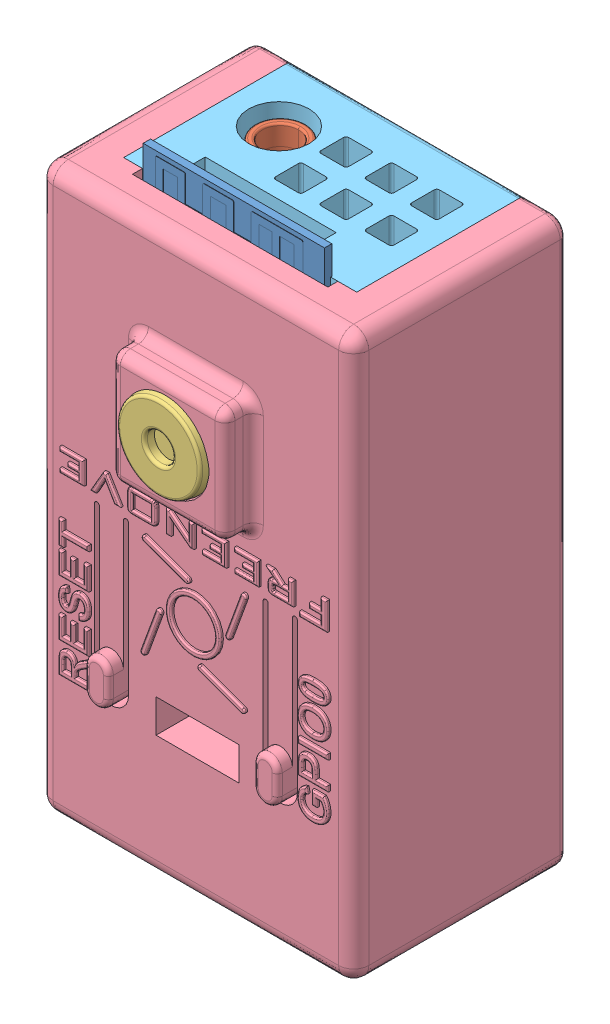
SolidWorks assembly FNK0102_Assembly_No_Battery, configuration 默认. Lengths in mm.
Overall size (31.34 58.7 30.41).
5 component instances, 5 part files, 10 mates.
Components (placement in the parent):
- CB8201_20250427-1: CB8201_20250427 [默认] at (-3.6296 -20.6055 14.3314) x (1 0 0) z (0 0 1) size (27.94 57.2 13.09)
- CB10201-1: CB10201 [默认] at (17.1633 5.4788 -53.4541) size (27.94 53.02 18.11)
- Camera_OV3660-1: Camera_OV3660 [默认] at (10.5364 16.4245 16.8) size (13.1 21.9 8.2)
- FNK0102_Part1_v1.3-1: FNK0102_Part1_v1.3 [一体按键0.00间距] at (-3.6115 -20.6055 14.5) size (31.34 55.9 24)
- FNK0102_Part2_v1.3-1: FNK0102_Part2_v1.3 [0.0间距] at (-3.6115 30.1945 0) size (28.34 54.9 17.1)
Mates (geometry in assembly coordinates):
- 重合1: coincident: plane of assembly through (0 0 0) normal (0 0 1); plane of CB10201-1 through (-3.6296 -20.6055 0) normal (0 0 -1); plane of assembly
- 重合38: coincident: plane of assembly; plane of assembly; plane of CB8201_20250427-1 through (-3.6448 -20.8607 10.1) normal (0 0 -1); plane of CB10201-1 through (-1.0896 -19.3355 10.1) normal (0 0 1)
- 重合39: coincident: plane of assembly; plane of assembly; plane of CB8201_20250427-1 through (-3.4648 -20.6055 12.8952) normal (0 -1 0); plane of CB10201-1 through (-3.6296 -20.6055 10.1) normal (0 -1 0)
- 重合40: coincident: plane of assembly; plane of assembly; plane of CB8201_20250427-1 through (-3.6296 -18.2303 12.8752) normal (-1 0 0); plane of CB10201-1 through (-3.6296 -18.0655 10.1) normal (-1 0 0)
- 重合41: coincident: plane of assembly; plane of assembly; plane of CB10201-1 through (-3.6296 -20.6055 0) normal (0 0 -1); plane of FNK0102_Part2_v1.3-1 through (-3.6115 30.1945 0) normal (0 0 1)
- 重合43: coincident: plane of assembly; plane of assembly; plane of CB10201-1 through (24.3104 30.1945 0) normal (0 1 0); plane of FNK0102_Part2_v1.3-1 through (-3.8115 30.1945 -30.8432) normal (0 -1 0)
- 锁定1: lock: unknown of CB10201-1; unknown of FNK0102_Part2_v1.3-1
- 重合45: coincident: plane of assembly; plane of assembly; plane of FNK0102_Part1_v1.3-1 through (-3.6115 -20.6055 -2.3) normal (0 0 -1); plane of FNK0102_Part2_v1.3-1 through (-3.6115 30.1945 -2.3) normal (0 0 -1)
- 同心1: concentric: cylinder of assembly; cylinder of assembly; cylinder of FNK0102_Part1_v1.3-1 through (-0.8115 32.3945 -6.0577) axis (0 0 1) radius 0.4; cylinder of FNK0102_Part2_v1.3-1 through (-0.8115 32.3945 -6.0577) axis (0 0 -1) radius 0.4
- 重合46: coincident: plane of assembly; plane of assembly; plane of FNK0102_Part1_v1.3-1 through (-3.8115 33.5945 18.9) normal (1 0 0); plane of FNK0102_Part2_v1.3-1 through (-3.8115 30.1945 -2.3) normal (-1 0 0)
